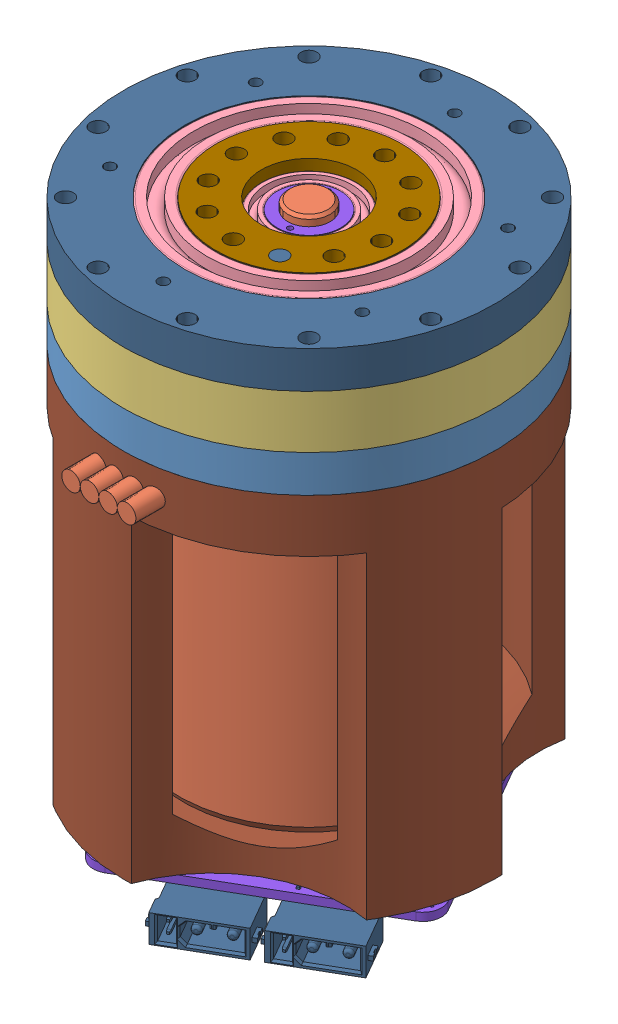
SolidWorks assembly Cycloidal_5065, configuration Default. Lengths in mm.
Overall size (95.62 102.59 95.62).
212 component instances, 82 part files, 54 mates.
Components (placement in the parent):
- Motor_base_5065-1: Motor_base_5065 [Default] at (25.1788 43.6468 54.8039) size (70 7 70)
- Flipsky 270kV motor.stp-1: Flipsky 270kV motor.stp [Default] at (25.1788 -19.3532 54.8039) x (0 1 0) z (-0.707107 0 0.707107) size (90.7 57.87 57.75)
- Ring_pin_housing_5065-1: Ring_pin_housing_5065 [Default] at (25.1788 50.6468 54.8039) size (70 10 70)
- radial ball bearing_68_iso-1: radial ball bearing_68_iso [ISO 15 RBB - 378 - 20,SI,NC,20_68] at (25.1788 48.8968 54.8039) x (0 1 0) z (-0.19787 0 0.980228) size (3.5 12 12)
- Ring_pin_5065-1: Ring_pin_5065 [Default] at (53.0279 61.6863 57.7576) x (-0.997886 0 0.064993) z (0.064993 0 0.997886) size (13.84 14 13.84)
  - m2_pin-1: m2_pin [Default] at (4.7265 1.0395 10.5113) size (4 14 4)
  - Ball_bearing_4x10x4-1: Ball_bearing_4x10x4 [Default] at (4.7265 9.0395 10.5113) size (10 4 10)
  - Ball_bearing_4x10x4-2: Ball_bearing_4x10x4 [Default] at (4.7265 3.0395 10.5113) x (-0.837169 0 -0.546944) z (-0.546944 0 0.837169) size (10 4 10)
- Ring_pin_5065-2: Ring_pin_5065 [Default] at (53.721 61.6863 30.5426) x (-1 0 0) z (0 0 1) size (13.84 14 13.84)
  - m2_pin-1: m2_pin [Default] at (4.7265 1.0395 10.5113) size (4 14 4)
  - Ball_bearing_4x10x4-1: Ball_bearing_4x10x4 [Default] at (4.7265 9.0395 10.5113) size (10 4 10)
  - Ball_bearing_4x10x4-2: Ball_bearing_4x10x4 [Default] at (4.7265 3.0395 10.5113) x (-0.837169 0 -0.546944) z (-0.546944 0 0.837169) size (10 4 10)
- Ring_pin_5065-3: Ring_pin_5065 [Default] at (15.4727 61.6863 76.0894) x (-0.146403 0 0.989225) z (0.989225 0 0.146403) size (13.84 14 13.84)
  - m2_pin-1: m2_pin [Default] at (4.7265 1.0395 10.5113) size (4 14 4)
  - Ball_bearing_4x10x4-1: Ball_bearing_4x10x4 [Default] at (4.7265 9.0395 10.5113) size (10 4 10)
  - Ball_bearing_4x10x4-2: Ball_bearing_4x10x4 [Default] at (4.7265 3.0395 10.5113) x (-0.837169 0 -0.546944) z (-0.546944 0 0.837169) size (10 4 10)
- Ring_pin_5065-4: Ring_pin_5065 [Default] at (6.0896 61.6863 58.0426) x (-1 0 0) z (0 0 1) size (13.84 14 13.84)
  - m2_pin-1: m2_pin [Default] at (4.7265 1.0395 10.5113) size (4 14 4)
  - Ball_bearing_4x10x4-1: Ball_bearing_4x10x4 [Default] at (4.7265 9.0395 10.5113) size (10 4 10)
  - Ball_bearing_4x10x4-2: Ball_bearing_4x10x4 [Default] at (4.7265 3.0395 10.5113) x (-0.837169 0 -0.546944) z (-0.546944 0 0.837169) size (10 4 10)
- Ring_pin_5065-5: Ring_pin_5065 [Default] at (29.9053 61.6863 16.7926) x (-1 0 0) z (0 0 1) size (13.84 14 13.84)
  - m2_pin-1: m2_pin [Default] at (4.7265 1.0395 10.5113) size (4 14 4)
  - Ball_bearing_4x10x4-1: Ball_bearing_4x10x4 [Default] at (4.7265 9.0395 10.5113) size (10 4 10)
  - Ball_bearing_4x10x4-2: Ball_bearing_4x10x4 [Default] at (4.7265 3.0395 10.5113) x (-0.837169 0 -0.546944) z (-0.546944 0 0.837169) size (10 4 10)
- Ring_pin_5065-6: Ring_pin_5065 [Default] at (6.0896 61.6863 30.5426) x (-1 0 0) z (0 0 1) size (13.84 14 13.84)
  - m2_pin-1: m2_pin [Default] at (4.7265 1.0395 10.5113) size (4 14 4)
  - Ball_bearing_4x10x4-1: Ball_bearing_4x10x4 [Default] at (4.7265 9.0395 10.5113) size (10 4 10)
  - Ball_bearing_4x10x4-2: Ball_bearing_4x10x4 [Default] at (4.7265 3.0395 10.5113) x (-0.837169 0 -0.546944) z (-0.546944 0 0.837169) size (10 4 10)
- Eccentric_shaft_5065-1: Eccentric_shaft_5065 [Default] at (16.4306 47.0254 47.869) x (0.967578 0 -0.252572) z (0.252572 0 0.967578) size (14 15 12)
  - Eccentric_shaft_bot_5065-1: Eccentric_shaft_bot_5065 [Default] at (6.713 3.6214 8.9195) size (12 5 12)
  - Eccentric_shaft_top_5065-1: Eccentric_shaft_top_5065 [Default] at (6.713 13.6214 8.9195) size (12 5 12)
  - Eccentric_shaft_bot_5065-2: Eccentric_shaft_bot_5065 [Default] at (6.713 8.6214 8.9195) x (-1 0 0) z (0 0 -1) size (12 5 12)
- radial ball bearing_68_iso-2: radial ball bearing_68_iso [ISO 15 RBB - 1712 - 20,SI,NC,20_68] at (25.1788 63.6468 54.8039) x (0 1 0) z (0 0 1) size (4 18 18)
- radial ball bearing_68_iso-3: radial ball bearing_68_iso [ISO 15 RBB - 1712 - 20,SI,NC,20_68] at (26.1463 58.6468 54.5513) x (0 -1 0) z (0.979558 0 -0.201164) size (4 18 18)
- radial ball bearing_68_iso-4: radial ball bearing_68_iso [ISO 15 RBB - 1712 - 20,SI,NC,20_68] at (24.2112 53.6468 55.0564) x (0 1 0) z (0 0 1) size (4 18 18)
- OutPut_shaft_5065-1: OutPut_shaft_5065 [Default] at (25.1788 60.6468 54.8039) x (0.876098 0 -0.482134) z (0.482134 0 0.876098) size (35 7 35)
- Output_cover_5065-1: Output_cover_5065 [Default] at (25.1788 60.6468 54.8039) size (70 7 70)
- Motor_cover_5065-1: Motor_cover_5065 [Default] at (25.1788 43.6468 54.8039) x (-0.866025 0 0.5) z (0.5 0 0.866025) size (70 70 70)
- Cycloidal_discs_5065-3: Cycloidal_discs_5065 [Default] at (3.9569 27.0207 21.2343) x (0.99705 0 -0.076752) z (0.076752 0 0.99705) size (45.09 5 45.95)
  - Cycloidal_discs_5065-1: Cycloidal_discs_5065 [Default] at (17.5986 23.6261 35.277) size (45.09 5 45.95)
  - radial ball bearing_68_iso-1: radial ball bearing_68_iso [ISO 15 RBB - 274 - 14,SI,NC,14_68] at (10.5986 27.3761 23.1526) x (0 1 0) z (-0.544662 0 0.838655) size (2.5 7 7)
  - radial ball bearing_68_iso-2: radial ball bearing_68_iso [ISO 15 RBB - 274 - 14,SI,NC,14_68] at (24.5986 27.3761 23.1526) x (0 1 0) z (-0.544662 0 0.838655) size (2.5 7 7)
  - radial ball bearing_68_iso-3: radial ball bearing_68_iso [ISO 15 RBB - 274 - 14,SI,NC,14_68] at (31.5986 27.3761 35.277) x (0 1 0) z (-0.544662 0 0.838655) size (2.5 7 7)
  - radial ball bearing_68_iso-4: radial ball bearing_68_iso [ISO 15 RBB - 274 - 14,SI,NC,14_68] at (24.5986 27.3761 47.4013) x (0 1 0) z (-0.544662 0 0.838655) size (2.5 7 7)
  - radial ball bearing_68_iso-5: radial ball bearing_68_iso [ISO 15 RBB - 274 - 14,SI,NC,14_68] at (10.5986 27.3761 47.4013) x (0 1 0) z (-0.544662 0 0.838655) size (2.5 7 7)
  - radial ball bearing_68_iso-6: radial ball bearing_68_iso [ISO 15 RBB - 274 - 14,SI,NC,14_68] at (3.5986 27.3761 35.277) x (0 1 0) z (-0.544662 0 0.838655) size (2.5 7 7)
- Cycloidal_discs_5065-5: Cycloidal_discs_5065 [Default] at (64.9013 32.0207 61.778) x (-0.602874 0 0.797837) z (-0.797837 0 -0.602874) size (45.09 5 45.95)
  - Cycloidal_discs_5065-1: Cycloidal_discs_5065 [Default] at (17.5986 23.6261 35.277) size (45.09 5 45.95)
  - radial ball bearing_68_iso-1: radial ball bearing_68_iso [ISO 15 RBB - 274 - 14,SI,NC,14_68] at (10.5986 27.3761 23.1526) x (0 1 0) z (-0.544662 0 0.838655) size (2.5 7 7)
  - radial ball bearing_68_iso-2: radial ball bearing_68_iso [ISO 15 RBB - 274 - 14,SI,NC,14_68] at (24.5986 27.3761 23.1526) x (0 1 0) z (-0.544662 0 0.838655) size (2.5 7 7)
  - radial ball bearing_68_iso-3: radial ball bearing_68_iso [ISO 15 RBB - 274 - 14,SI,NC,14_68] at (31.5986 27.3761 35.277) x (0 1 0) z (-0.544662 0 0.838655) size (2.5 7 7)
  - radial ball bearing_68_iso-4: radial ball bearing_68_iso [ISO 15 RBB - 274 - 14,SI,NC,14_68] at (24.5986 27.3761 47.4013) x (0 1 0) z (-0.544662 0 0.838655) size (2.5 7 7)
  - radial ball bearing_68_iso-5: radial ball bearing_68_iso [ISO 15 RBB - 274 - 14,SI,NC,14_68] at (10.5986 27.3761 47.4013) x (0 1 0) z (-0.544662 0 0.838655) size (2.5 7 7)
  - radial ball bearing_68_iso-6: radial ball bearing_68_iso [ISO 15 RBB - 274 - 14,SI,NC,14_68] at (3.5986 27.3761 35.277) x (0 1 0) z (-0.544662 0 0.838655) size (2.5 7 7)
- radial ball bearing_68_iso-5: radial ball bearing_68_iso [ISO 15 RBB - 274 - 14,SI,NC,14_68] at (25.1788 51.8968 54.8039) x (0 1 0) z (0.001306 0 0.999999) size (2.5 7 7)
- foc-motor-controller.step-1: foc-motor-controller.step [Default] at (25.1788 -28.1532 54.8039) x (-0.5 0 -0.866025) z (0 -1 0) size (57.23 50 8.13)
  - RTA0040B.step-1: RTA0040B.step [Default] at (12.5014 -1.6986 1.595) x (-0.707107 -0.707107 0) z (0 0 1) size (6 6 1)
    - FRAME.step-1: FRAME.step [Default] x (1 0 0) z (0 -1 0) size (6 0.2 6)
      - SOLID.step-1: SOLID.step [Default] at origin size (0.4 0.2 0.22)
      - SOLID-0.step-1: SOLID-0.step [Default] at origin size (0.4 0.2 0.22)
      - SOLID-1.step-1: SOLID-1.step [Default] at origin size (0.4 0.2 0.22)
      - SOLID-2.step-1: SOLID-2.step [Default] at origin size (0.4 0.2 0.22)
      - SOLID-3.step-1: SOLID-3.step [Default] at origin size (0.4 0.2 0.22)
      - SOLID-4.step-1: SOLID-4.step [Default] at origin size (0.4 0.2 0.22)
      - SOLID-5.step-1: SOLID-5.step [Default] at origin size (0.4 0.2 0.22)
      - SOLID-6.step-1: SOLID-6.step [Default] at origin size (0.4 0.2 0.22)
      - SOLID-7.step-1: SOLID-7.step [Default] at origin size (0.4 0.2 0.22)
      - SOLID-8.step-1: SOLID-8.step [Default] at origin size (0.4 0.2 0.22)
      - SOLID-9.step-1: SOLID-9.step [Default] at origin size (0.22 0.2 0.4)
      - SOLID-10.step-1: SOLID-10.step [Default] at origin size (0.22 0.2 0.4)
      - SOLID-11.step-1: SOLID-11.step [Default] at origin size (0.22 0.2 0.4)
      - SOLID-12.step-1: SOLID-12.step [Default] at origin size (0.22 0.2 0.4)
      - SOLID-13.step-1: SOLID-13.step [Default] at origin size (0.22 0.2 0.4)
      - SOLID-14.step-1: SOLID-14.step [Default] at origin size (0.22 0.2 0.4)
      - SOLID-15.step-1: SOLID-15.step [Default] at origin size (0.22 0.2 0.4)
      - SOLID-16.step-1: SOLID-16.step [Default] at origin size (0.22 0.2 0.4)
      - SOLID-17.step-1: SOLID-17.step [Default] at origin size (4.15 0.2 4.15)
      - SOLID-18.step-1: SOLID-18.step [Default] at origin size (0.28 0.1 0.28)
      - SOLID-19.step-1: SOLID-19.step [Default] at origin size (0.28 0.1 0.28)
      - SOLID-20.step-1: SOLID-20.step [Default] at origin size (0.28 0.1 0.28)
      - SOLID-21.step-1: SOLID-21.step [Default] at origin size (0.28 0.1 0.28)
      - SOLID-22.step-1: SOLID-22.step [Default] at origin size (0.4 0.2 0.22)
      - SOLID-23.step-1: SOLID-23.step [Default] at origin size (0.4 0.2 0.22)
      - SOLID-24.step-1: SOLID-24.step [Default] at origin size (0.4 0.2 0.22)
      - SOLID-25.step-1: SOLID-25.step [Default] at origin size (0.4 0.2 0.22)
      - SOLID-26.step-1: SOLID-26.step [Default] at origin size (0.4 0.2 0.22)
      - SOLID-27.step-1: SOLID-27.step [Default] at origin size (0.4 0.2 0.22)
      - SOLID-28.step-1: SOLID-28.step [Default] at origin size (0.4 0.2 0.22)
      - SOLID-29.step-1: SOLID-29.step [Default] at origin size (0.4 0.2 0.22)
      - SOLID-30.step-1: SOLID-30.step [Default] at origin size (0.4 0.2 0.22)
      - SOLID-31.step-1: SOLID-31.step [Default] at origin size (0.4 0.2 0.22)
      - SOLID-32.step-1: SOLID-32.step [Default] at origin size (0.22 0.2 0.4)
      - SOLID-33.step-1: SOLID-33.step [Default] at origin size (0.22 0.2 0.4)
      - SOLID-34.step-1: SOLID-34.step [Default] at origin size (0.22 0.2 0.4)
      - SOLID-35.step-1: SOLID-35.step [Default] at origin size (0.22 0.2 0.4)
      - SOLID-36.step-1: SOLID-36.step [Default] at origin size (0.22 0.2 0.4)
      - SOLID-37.step-1: SOLID-37.step [Default] at origin size (0.22 0.2 0.4)
      - SOLID-38.step-1: SOLID-38.step [Default] at origin size (0.22 0.2 0.4)
      - SOLID-39.step-1: SOLID-39.step [Default] at origin size (0.22 0.2 0.4)
      - SOLID-40.step-1: SOLID-40.step [Default] at origin size (0.22 0.2 0.4)
      - SOLID-41.step-1: SOLID-41.step [Default] at origin size (0.22 0.2 0.4)
      - SOLID-42.step-1: SOLID-42.step [Default] at origin size (0.22 0.2 0.4)
      - SOLID-43.step-1: SOLID-43.step [Default] at origin size (0.22 0.2 0.4)
    - BODY.step-1: BODY.step [Default] at (0 0 0.025) x (1 0 0) z (0 -1 0) size (6 0.97 6)
  - Resonator_SMD_Murata_CSTxExxV-3Pin_3.0x1.1mm.step-1: Resonator_SMD_Murata_CSTxExxV-3Pin_3.0x1.1mm.step [Default] at (1.8 -7 1.595) x (0 1 0) z (0 0 1) size (3.2 1.35 0.9)
  - C_0603_1608Metric.step-1: C_0603_1608Metric.step [Default] at (6.2 -16.8 1.595) x (0 -1 0) z (0 0 1) size (1.6 0.8 0.8)
  - R_0603_1608Metric.step-1: R_0603_1608Metric.step [Default] at (11.8 -7.375 1.595) x (0 1 0) z (0 0 1) size (1.6 0.8 0.45)
  - R_0603_1608Metric.step-2: R_0603_1608Metric.step [Default] at (13.8 -16.8 1.595) x (0 1 0) z (0 0 1) size (1.6 0.8 0.45)
  - R_0603_1608Metric.step-3: R_0603_1608Metric.step [Default] at (18.1 -5.36 1.595) size (1.6 0.8 0.45)
  - C_0603_1608Metric.step-2: C_0603_1608Metric.step [Default] at (2.6 -0.5 1.595) x (0 -1 0) z (0 0 1) size (1.6 0.8 0.8)
  - R_0603_1608Metric.step-4: R_0603_1608Metric.step [Default] at (14.6 -11.3 1.595) x (0 1 0) z (0 0 1) size (1.6 0.8 0.45)
  - L_APV_ANR4020.step-1: L_APV_ANR4020.step [Default] at (22.3 -13.7 1.595) x (0 -1 0) z (0 0 1) size (4.02 4 2)
  - C_0603_1608Metric.step-3: C_0603_1608Metric.step [Default] at (0.3 -12.6 1.595) x (-1 0 0) z (0 0 1) size (1.6 0.8 0.8)
  - C_1206_3216Metric.step-1: C_1206_3216Metric.step [Default] at (15.7 11 1.595) x (0 1 0) z (0 0 1) size (3.2 1.6 1.6)
  - C_0603_1608Metric.step-4: C_0603_1608Metric.step [Default] at (0.3 -9.6 1.595) size (1.6 0.8 0.8)
  - R_0603_1608Metric.step-5: R_0603_1608Metric.step [Default] at (12.3 -16.8 1.595) x (0 1 0) z (0 0 1) size (1.6 0.8 0.45)
  - C_0603_1608Metric.step-5: C_0603_1608Metric.step [Default] at (-0.3 -16.6 1.595) x (0 1 0) z (0 0 1) size (1.6 0.8 0.8)
  - R_0603_1608Metric.step-6: R_0603_1608Metric.step [Default] at (10.9 4.1 1.595) size (1.6 0.8 0.45)
  - C_1206_3216Metric.step-2: C_1206_3216Metric.step [Default] at (6.3 11 1.595) x (0 1 0) z (0 0 1) size (3.2 1.6 1.6)
  - XT30PW_2_2_-M.G.B.step-1: XT30PW_2_2_-M.G.B.step [Default] at (-20.5 9.5 1.595) x (0 -1 0) z (-1 0 0) size (15.5 7.1 12.53)
  - R_0603_1608Metric.step-7: R_0603_1608Metric.step [Default] at (0.3 -11.1 1.595) size (1.6 0.8 0.45)
  - C_0603_1608Metric.step-6: C_0603_1608Metric.step [Default] at (19 -0.4 1.595) x (-0.707107 -0.707107 0) z (0 0 1) size (1.6 0.8 0.8)
  - C_1206_3216Metric.step-3: C_1206_3216Metric.step [Default] at (13.3 11 1.595) x (0 1 0) z (0 0 1) size (3.2 1.6 1.6)
  - R_0603_1608Metric.step-8: R_0603_1608Metric.step [Default] at (10.2 -7.375 1.595) x (0 -1 0) z (0 0 1) size (1.6 0.8 0.45)
  - JST_GH_SM08B-GHS-TB_1x08-1MP_P1.25mm_Horizontal.step-1: JST_GH_SM08B-GHS-TB_1x08-1MP_P1.25mm_Horizontal.step [Default] at (10 -22 1.595) size (13.25 4.95 4.25)
  - C_1206_3216Metric.step-4: C_1206_3216Metric.step [Default] at (-12.3 11 1.595) x (0 1 0) z (0 0 1) size (3.2 1.6 1.6)
  - JST_GH_SM06B-GHS-TB_1x06-1MP_P1.25mm_Horizontal.step-1: JST_GH_SM06B-GHS-TB_1x06-1MP_P1.25mm_Horizontal.step [Default] at (-4.3 -22 1.595) size (10.75 4.95 4.25)
  - C_0603_1608Metric.step-7: C_0603_1608Metric.step [Default] at (7.3 -4.5 1.595) x (-1 0 0) z (0 0 1) size (1.6 0.8 0.8)
  - R_0603_1608Metric.step-9: R_0603_1608Metric.step [Default] at (18.1 -3.86 1.595) x (-1 0 0) z (0 0 1) size (1.6 0.8 0.45)
  - C_1206_3216Metric.step-5: C_1206_3216Metric.step [Default] at (22.6794 -1.2206 1.595) x (0.707107 -0.707107 0) z (0 0 1) size (3.2 1.6 1.6)
  - R_Array_Convex_4x0402.step-1: R_Array_Convex_4x0402.step [Default] at (6.8 -2.5 1.595) size (1 2 0.35)
  - R_0603_1608Metric.step-10: R_0603_1608Metric.step [Default] at (7.7 -16.8 1.595) x (0 -1 0) z (0 0 1) size (1.6 0.8 0.45)
  - C_1206_3216Metric.step-6: C_1206_3216Metric.step [Default] at (8.7 11 1.595) x (0 1 0) z (0 0 1) size (3.2 1.6 1.6)
  - C_0603_1608Metric.step-8: C_0603_1608Metric.step [Default] at (16.1 -11.3 1.595) x (0 1 0) z (0 0 1) size (1.6 0.8 0.8)
  - SOT-23-5.step-1: SOT-23-5.step [Default] at (-3.1 -16.6 1.595) x (-1 0 0) z (0 0 1) size (2.8 2.9 1.55)
  - C_0603_1608Metric.step-9: C_0603_1608Metric.step [Default] at (17.8 -13.6 1.595) size (1.6 0.8 0.8)
  - R_0603_1608Metric.step-11: R_0603_1608Metric.step [Default] at (-11.5 -20.3875 1.595) x (0 -1 0) z (0 0 1) size (1.6 0.8 0.45)
  - C_0603_1608Metric.step-10: C_0603_1608Metric.step [Default] at (-12.4 2.3 1.595) x (0 1 0) z (0 0 1) size (1.6 0.8 0.8)
  - C_1206_3216Metric.step-7: C_1206_3216Metric.step [Default] at (18 11 1.595) x (0 1 0) z (0 0 1) size (3.2 1.6 1.6)
  - R_0603_1608Metric.step-12: R_0603_1608Metric.step [Default] at (-10.8105 -14.9971 1.595) x (-1 0 0) z (0 0 1) size (1.6 0.8 0.45)
  - C_0603_1608Metric.step-11: C_0603_1608Metric.step [Default] at (-13.8 -9.4 1.595) x (-1 0 0) z (0 0 1) size (1.6 0.8 0.8)
  - R_0603_1608Metric.step-13: R_0603_1608Metric.step [Default] at (-23.15 -14.5 1.595) x (-1 0 0) z (0 0 1) size (1.6 0.8 0.45)
  - C_0603_1608Metric.step-12: C_0603_1608Metric.step [Default] at (1.1 -0.2 1.595) x (0 1 0) z (0 0 1) size (1.6 0.8 0.8)
  - D_0805_2012Metric.step-1: D_0805_2012Metric.step [Default] at (22.9 -9.6 1.595) x (0 1 0) z (0 0 1) size (2 1.27 0.8)
  - C_0603_1608Metric.step-13: C_0603_1608Metric.step [Default] at (-7.8 3.775 1.595) x (0 -1 0) z (0 0 1) size (1.6 0.8 0.8)
  - R_0603_1608Metric.step-14: R_0603_1608Metric.step [Default] at (-6.4 -12.825 1.595) x (0 1 0) z (0 0 1) size (1.6 0.8 0.45)
  - L_0603_1608Metric.step-1: L_0603_1608Metric.step [Default] at (-10.1 3 1.595) size (1.6 0.8 0.8)
  - C_0603_1608Metric.step-14: C_0603_1608Metric.step [Default] at (17.9 0.7 1.595) x (-0.707107 -0.707107 0) z (0 0 1) size (1.6 0.8 0.8)
  - HVSSOP-10.step-1: HVSSOP-10.step [Default] at (18.6 -9.6 1.595) x (0 -1 0) z (-1 0 0) size (4.9 1.1 3)
  - C_0603_1608Metric.step-15: C_0603_1608Metric.step [Default] at (7.9 4.1 1.595) x (-1 0 0) z (0 0 1) size (1.6 0.8 0.8)
  - C_0603_1608Metric.step-16: C_0603_1608Metric.step [Default] at (21.1 -9.6 1.595) x (0 -1 0) z (0 0 1) size (1.6 0.8 0.8)
  - R_0603_1608Metric.step-15: R_0603_1608Metric.step [Default] at (-10.8105 -11.9971 1.595) x (-1 0 0) z (0 0 1) size (1.6 0.8 0.45)
  - R_0603_1608Metric.step-16: R_0603_1608Metric.step [Default] at (-18.2 -17.4 1.595) size (1.6 0.8 0.45)
  - C_1206_3216Metric.step-8: C_1206_3216Metric.step [Default] at (-3 11 1.595) x (0 1 0) z (0 0 1) size (3.2 1.6 1.6)
  - R_0603_1608Metric.step-17: R_0603_1608Metric.step [Default] at (-16.9 -20.4 1.595) x (0 -1 0) z (0 0 1) size (1.6 0.8 0.45)
  - R_0603_1608Metric.step-18: R_0603_1608Metric.step [Default] at (-13.3 -20.3875 1.595) x (0 -1 0) z (0 0 1) size (1.6 0.8 0.45)
  - R_0603_1608Metric.step-19: R_0603_1608Metric.step [Default] at (-15.1 -20.3875 1.595) x (0 -1 0) z (0 0 1) size (1.6 0.8 0.45)
  - C_0603_1608Metric.step-17: C_0603_1608Metric.step [Default] at (15.5 -14.4 1.595) x (0 -1 0) z (0 0 1) size (1.6 0.8 0.8)
  - LED_0603_1608Metric.step-1: LED_0603_1608Metric.step [Default] at (-11.5 -23.3875 1.595) x (0 1 0) z (0 0 1) size (1.6 0.8 1.1)
  - C_0805_2012Metric.step-1: C_0805_2012Metric.step [Default] at (19.95 -17 1.595) size (2 1.25 1.25)
  - D_SMB.step-1: D_SMB.step [Default] at (-16.5 11.208 1.595) x (0 -1 0) z (0 0 1) size (5.3 3.55 2.15)
  - C_1206_3216Metric.step-9: C_1206_3216Metric.step [Default] at (-5.3 11 1.595) x (0 1 0) z (0 0 1) size (3.2 1.6 1.6)
  - XT30PW_2_2_-M.G.B.step-2: XT30PW_2_2_-M.G.B.step [Default] at (-20.5 -6.5 1.595) x (0 -1 0) z (-1 0 0) size (15.5 7.1 12.53)
  - C_1206_3216Metric.step-10: C_1206_3216Metric.step [Default] at (1.7 11 1.595) x (0 1 0) z (0 0 1) size (3.2 1.6 1.6)
  - C_1206_3216Metric.step-11: C_1206_3216Metric.step [Default] at (11 11 1.595) x (0 1 0) z (0 0 1) size (3.2 1.6 1.6)
  - C_0603_1608Metric.step-18: C_0603_1608Metric.step [Default] at (-6.3 3.775 1.595) x (0 -1 0) z (0 0 1) size (1.6 0.8 0.8)
  - C_0603_1608Metric.step-19: C_0603_1608Metric.step [Default] at (16.8686 1.7314 1.595) x (0.707107 0.707107 0) z (0 0 1) size (1.6 0.8 0.8)
  - C_0603_1608Metric.step-20: C_0603_1608Metric.step [Default] at (-15.0105 -11.1 1.595) size (1.6 0.8 0.8)
  - C_1206_3216Metric.step-12: C_1206_3216Metric.step [Default] at (-7.7 11 1.595) x (0 1 0) z (0 0 1) size (3.2 1.6 1.6)
  - C_0603_1608Metric.step-21: C_0603_1608Metric.step [Default] at (-18.2 -15.8 1.595) size (1.6 0.8 0.8)
  - C_0603_1608Metric.step-22: C_0603_1608Metric.step [Default] at (-2.1 -11.3 1.595) x (0 -1 0) z (0 0 1) size (1.6 0.8 0.8)
  - C_0603_1608Metric.step-23: C_0603_1608Metric.step [Default] at (-10.8105 -13.4971 1.595) size (1.6 0.8 0.8)
  - C_1206_3216Metric.step-13: C_1206_3216Metric.step [Default] at (4 11 1.595) x (0 1 0) z (0 0 1) size (3.2 1.6 1.6)
  - R_0603_1608Metric.step-20: R_0603_1608Metric.step [Default] at (16 -17.8 1.595) x (0 1 0) z (0 0 1) size (1.6 0.8 0.45)
  - Texas_S-PVSON-N8.step-1: Texas_S-PVSON-N8.step [Default] at (-14.4105 -13.7 1.595) x (-1 0 0) z (0 0 1) size (3 2.98 0.92)
  - C_1206_3216Metric.step-14: C_1206_3216Metric.step [Default] at (21 -2.9 1.595) x (0.707107 -0.707107 0) z (0 0 1) size (3.2 1.6 1.6)
  - C_0603_1608Metric.step-24: C_0603_1608Metric.step [Default] at (-5.9 -16.6 1.595) x (0 1 0) z (0 0 1) size (1.6 0.8 0.8)
  - C_0603_1608Metric.step-25: C_0603_1608Metric.step [Default] at (-3.1 -14.1 1.595) size (1.6 0.8 0.8)
  - R_0603_1608Metric.step-21: R_0603_1608Metric.step [Default] at (7.2 -7.375 1.595) x (0 -1 0) z (0 0 1) size (1.6 0.8 0.45)
  - C_1206_3216Metric.step-15: C_1206_3216Metric.step [Default] at (-0.7 11 1.595) x (0 1 0) z (0 0 1) size (3.2 1.6 1.6)
  - LQFP-64_10x10mm_P0.5mm.step-1: LQFP-64_10x10mm_P0.5mm.step [Default] at (-7 -4.5 1.595) x (-1 0 0) z (0 0 1) size (12 12 1.5)
  - C_0805_2012Metric.step-2: C_0805_2012Metric.step [Default] at (23.35 -17 1.595) x (-1 0 0) z (0 0 1) size (2 1.25 1.25)
  - C_0603_1608Metric.step-26: C_0603_1608Metric.step [Default] at (10.8 -16.8 1.595) x (0 -1 0) z (0 0 1) size (1.6 0.8 0.8)
  - R_0603_1608Metric.step-22: R_0603_1608Metric.step [Default] at (17.5 -17.8 1.595) x (0 -1 0) z (0 0 1) size (1.6 0.8 0.45)
  - C_1206_3216Metric.step-16: C_1206_3216Metric.step [Default] at (20.3 11 1.595) x (0 1 0) z (0 0 1) size (3.2 1.6 1.6)
  - R_0603_1608Metric.step-23: R_0603_1608Metric.step [Default] at (9.2 -16.8 1.595) x (0 -1 0) z (0 0 1) size (1.6 0.8 0.45)
  - C_1206_3216Metric.step-17: C_1206_3216Metric.step [Default] at (-10 11 1.595) x (0 1 0) z (0 0 1) size (3.2 1.6 1.6)
  - R_0603_1608Metric.step-24: R_0603_1608Metric.step [Default] at (17.8 -15.2 1.595) size (1.6 0.8 0.45)
  - C_1206_3216Metric.step-18: C_1206_3216Metric.step [Default] at (19.9 2.6 1.595) x (-0.707107 0.707107 0) z (0 0 1) size (3.2 1.6 1.6)
  - C_0603_1608Metric.step-27: C_0603_1608Metric.step [Default] at (13.4 -7.375 1.595) x (0 -1 0) z (0 0 1) size (1.6 0.8 0.8)
  - R_0603_1608Metric.step-25: R_0603_1608Metric.step [Default] at (8.7 -7.375 1.595) x (0 -1 0) z (0 0 1) size (1.6 0.8 0.45)
  - PQFN-8-EP_6x5mm_P1.27mm_Generic.step-1: PQFN-8-EP_6x5mm_P1.27mm_Generic.step [Default] at (4.9 14.4 -0.085) x (0 1 0) z (0 0 -1) size (6.15 5.15 1.09)
  - C_0805_2012Metric.step-3: C_0805_2012Metric.step [Default] at (-3 8.9 -0.085) x (0 1 0) z (0 0 -1) size (2 1.25 1.25)
  - C_0603_1608Metric.step-28: C_0603_1608Metric.step [Default] at (1.5 -4.3 -0.085) x (0 1 0) z (0 0 -1) size (1.6 0.8 0.8)
  - R_2512_6332Metric.step-1: R_2512_6332Metric.step [Default] at (2.1 8.6 -0.085) x (-1 0 0) z (0 0 -1) size (6.3 3.2 0.6)
  - C_0805_2012Metric.step-4: C_0805_2012Metric.step [Default] at (18.8 8.9 -0.085) x (0 1 0) z (0 0 -1) size (2 1.25 1.25)
  - C_0805_2012Metric.step-5: C_0805_2012Metric.step [Default] at (-5.2 8.901 -0.085) x (0 1 0) z (0 0 -1) size (2 1.25 1.25)
  - PQFN-8-EP_6x5mm_P1.27mm_Generic.step-2: PQFN-8-EP_6x5mm_P1.27mm_Generic.step [Default] at (16.9 14.6 -0.085) x (0 -1 0) z (0 0 -1) size (6.15 5.15 1.09)
  - PQFN-8-EP_6x5mm_P1.27mm_Generic.step-3: PQFN-8-EP_6x5mm_P1.27mm_Generic.step [Default] at (-1.1 14.6 -0.085) x (0 -1 0) z (0 0 -1) size (6.15 5.15 1.09)
  - R_0603_1608Metric.step-26: R_0603_1608Metric.step [Default] at (8.2 8.8 -0.085) x (0 1 0) z (0 0 -1) size (1.6 0.8 0.45)
  - R_2512_6332Metric.step-2: R_2512_6332Metric.step [Default] at (-10.3 8.601 -0.085) x (1 0 0) z (0 0 -1) size (6.3 3.2 0.6)
  - TSSOP-16_4.4x5mm_P0.65mm.step-1: TSSOP-16_4.4x5mm_P0.65mm.step [Default] at (0 0 -0.085) x (-1 0 0) z (0 0 -1) size (6.4 5 1.1)
  - C_0603_1608Metric.step-29: C_0603_1608Metric.step [Default] at (0 -4.25 -0.085) x (0 1 0) z (0 0 -1) size (1.6 0.8 0.8)
  - PQFN-8-EP_6x5mm_P1.27mm_Generic.step-4: PQFN-8-EP_6x5mm_P1.27mm_Generic.step [Default] at (10.9 14.4 -0.085) x (0 1 0) z (0 0 -1) size (6.15 5.15 1.09)
  - R_2512_6332Metric.step-3: R_2512_6332Metric.step [Default] at (13.7 8.6 -0.085) x (1 0 0) z (0 0 -1) size (6.3 3.2 0.6)
  - PQFN-8-EP_6x5mm_P1.27mm_Generic.step-5: PQFN-8-EP_6x5mm_P1.27mm_Generic.step [Default] at (-13.1 14.401 -0.085) x (0 1 0) z (0 0 -1) size (6.15 5.15 1.09)
  - C_0603_1608Metric.step-30: C_0603_1608Metric.step [Default] at (-1.5 -4.3 -0.085) x (0 -1 0) z (0 0 -1) size (1.6 0.8 0.8)
  - PQFN-8-EP_6x5mm_P1.27mm_Generic.step-6: PQFN-8-EP_6x5mm_P1.27mm_Generic.step [Default] at (-7.1 14.601 -0.085) x (0 -1 0) z (0 0 -1) size (6.15 5.15 1.09)
  - foc-motor-controller_PCB.step-1: foc-motor-controller_PCB.step [Default] at origin size (50 50 1.51)
- hex thin nut chamfered gradeab_iso-1: hex thin nut chamfered gradeab_iso [PreviewCfg] at (33.0483 -26.3532 25.4343) x (0.517651 0 -0.855592) z (0 1 0) size (5.5 6.35 1.8)
- m3_5065-1: m3_5065 [Default] at (31.9286 50.6468 67.0692) size (3 17 3)
- radial ball bearing_68_iso-7: radial ball bearing_68_iso [ISO 15 RBB - 1835 - 28,SI,NC,28_68] at (25.1788 64.1468 54.8039) x (0 1 0) z (0 0 1) size (7 47 47)
Mates (geometry in assembly coordinates):
- Coincident1: coincident anti-aligned: plane of Motor_base_5065-1 through (25.1788 43.6468 54.8039) normal (0 -1 0); plane of Flipsky 270kV motor.stp-1 through (25.1788 43.6468 54.8039) normal (0 1 0)
- Concentric1: concentric aligned: cylinder of Motor_base_5065-1 through (25.1788 50.6468 54.8039) axis (0 -1 0) radius 6; cylinder of Flipsky 270kV motor.stp-1 through (25.1788 43.6468 54.8039) axis (0 -1 0) radius 4
- Parallel1: parallel aligned: cylinder of Motor_base_5065-1 through (2.1978 50.6468 77.7848) axis (0 -1 0) radius 1.5; cylinder of Ring_pin_housing-1 through (2.1978 60.6468 77.7848) axis (0 -1 0) radius 1.5
- Concentric4: concentric aligned: cylinder of Motor_base_5065-1 through (1.3631 50.6468 68.5539) axis (0 -1 0) radius 1; cylinder of Ring_pin_housing-1 through (1.3631 60.6468 68.5539) axis (0 -1 0) radius 5.5
- Concentric5: concentric anti-aligned: cylinder of Motor_base_5065-1 through (25.1788 50.6468 54.8039) axis (0 -1 0) radius 6; cylinder of radial ball bearing_68_iso-1 through (25.1788 28.2593 54.8039) axis (0 1 0) radius 4
- Concentric6: concentric anti-aligned: cylinder of Motor_base_5065-1 through (48.9945 50.6468 68.5539) axis (0 -1 0) radius 1; cylinder of Ring_pin-1/m2_pin-1 through (48.9945 46.6468 68.5539) axis (0 1 0) radius 1
- Coincident3: coincident anti-aligned: plane of Motor_base_5065-1 through (25.1788 50.6468 54.8039) normal (0 1 0); plane of Ring_pin_5065-1/Ball_bearing_4x10x4-1 through (48.9945 50.6468 68.5539) normal (0 -1 0)
- Concentric7: concentric anti-aligned: cylinder of Motor_base_5065-1 through (48.9945 50.6468 41.0539) axis (0 -1 0) radius 1; cylinder of Ring_pin-2/m2_pin-1 through (48.9945 46.6468 41.0539) axis (0 1 0) radius 1
- Coincident4: coincident anti-aligned: plane of Motor_base_5065-1 through (25.1788 50.6468 54.8039) normal (0 1 0); plane of Ring_pin-2/Ball_bearing_4x10x4-1 through (48.9945 50.6468 41.0539) normal (0 -1 0)
- Coincident5: coincident anti-aligned: plane of Motor_base_5065-1 through (25.1788 50.6468 54.8039) normal (0 1 0); plane of Ring_pin_housing_5065-1 through (25.1788 50.6468 54.8039) normal (0 -1 0)
- Concentric9: concentric anti-aligned: cylinder of Motor_base_5065-1 through (25.1788 50.6468 82.3039) axis (0 -1 0) radius 1; cylinder of Ring_pin_5065-3/m2_pin-1 through (25.1788 46.6468 82.3039) axis (0 1 0) radius 1
- Concentric26: concentric anti-aligned: line of Motor_base_5065-1 through (25.1788 50.6468 27.3039) axis (0 -1 0); cylinder of Ring_pin-5/m2_pin-1 through (25.1788 50.6468 27.3039) axis (0 1 0) radius 1
- Concentric11: concentric anti-aligned: cylinder of Motor_base_5065-1 through (1.3631 50.6468 41.0539) axis (0 -1 0) radius 1; cylinder of Ring_pin-6/m2_pin-1 through (1.3631 46.6468 41.0539) axis (0 1 0) radius 1
- Concentric12: concentric anti-aligned: cylinder of Motor_base_5065-1 through (1.3631 50.6468 68.5539) axis (0 -1 0) radius 1; cylinder of Ring_pin-4/m2_pin-1 through (1.3631 46.6468 68.5539) axis (0 1 0) radius 1
- Coincident8: coincident anti-aligned: plane of Motor_base_5065-1 through (25.1788 50.6468 54.8039) normal (0 1 0); plane of Ring_pin-4/Ball_bearing_4x10x4-1 through (1.3631 50.6468 68.5539) normal (0 -1 0)
- Coincident9: coincident anti-aligned: plane of Motor_base_5065-1 through (25.1788 50.6468 54.8039) normal (0 1 0); plane of Ring_pin-6/Ball_bearing_4x10x4-1 through (1.3631 50.6468 41.0539) normal (0 -1 0)
- Coincident10: coincident anti-aligned: plane of Motor_base_5065-1 through (25.1788 50.6468 54.8039) normal (0 1 0); plane of Ring_pin-5/Ball_bearing_4x10x4-1 through (25.1788 50.6468 27.3039) normal (0 -1 0)
- Coincident11: coincident anti-aligned: plane of Motor_base_5065-1 through (25.1788 50.6468 54.8039) normal (0 1 0); plane of Eccentric_shaft_5065-1/Eccentric_shaft_bot_5065-1 through (24.2112 50.6468 55.0564) normal (0 -1 0)
- Concentric13: concentric anti-aligned: cylinder of radial ball bearing_68_iso-1 through (25.1788 28.2593 54.8039) axis (0 1 0) radius 4; cylinder of Eccentric_shaft_5065-1/Eccentric_shaft_bot_5065-2 through (25.1788 60.6468 54.8039) axis (0 -1 0) radius 4
- Concentric14: concentric anti-aligned: cylinder of Eccentric_shaft_5065-1/Eccentric_shaft_bot_5065-1 through (24.2112 55.6468 55.0564) axis (0 -1 0) radius 6; cylinder of radial ball bearing_68_iso-4 through (24.2112 33.0093 55.0564) axis (0 1 0) radius 6
- Coincident12: coincident aligned: plane of Eccentric_shaft_5065-1/Eccentric_shaft_bot_5065-1 through (24.2112 55.6468 55.0564) normal (0 1 0); circle of radial ball bearing_68_iso-4
- Concentric15: concentric anti-aligned: cylinder of ? through (26.1463 60.6468 54.5513) axis (0 -1 0) radius 6; line of radial ball bearing_68_iso-3 through (26.1463 54.0645 54.5513) axis (0 1 0)
- Coincident13: coincident aligned: circle of Eccentric_shaft-1/Eccentric_shaft_bot-2; plane of radial ball bearing_68_iso-3 through (24.7583 60.6468 47.7923) normal (0 1 0)
- Coincident14: coincident aligned: plane of Eccentric_shaft_5065-1/Eccentric_shaft_top_5065-1 through (25.1788 65.6468 54.8039) normal (0 1 0); circle of radial ball bearing_68_iso-2
- Concentric17: concentric anti-aligned: cylinder of Eccentric_shaft_5065-1/Eccentric_shaft_bot_5065-1 through (25.1788 55.6468 54.8039) axis (0 -1 0) radius 4; cylinder of radial ball bearing_68_iso-2 through (25.1788 43.0093 54.8039) axis (0 1 0) radius 6
- Concentric21: concentric anti-aligned: cylinder of radial ball bearing_68_iso-2 through (25.1788 43.0093 54.8039) axis (0 1 0) radius 9; cylinder of OutPut_shaft_5065-1 through (25.1788 67.6468 54.8039) axis (0 -1 0) radius 9
- Coincident20: coincident aligned: plane of Ring_pin_housing_5065-1 through (25.1788 60.6468 54.8039) normal (0 1 0); circle of Output_cover_5065-1
- Concentric24: concentric aligned: cylinder of Ring_pin_housing-1 through (2.1978 60.6468 77.7848) axis (0 -1 0) radius 1.5; cylinder of Output_cover_5065-1 through (2.1978 67.6468 77.7848) axis (0 -1 0) radius 1.5
- Coincident33: coincident aligned: plane of OutPut_shaft_5065-1 through (25.1788 67.6468 54.8039) normal (0 1 0); plane of Output_cover_5065-1 through (25.1788 67.6468 54.8039) normal (0 1 0)
- Concentric27: concentric aligned: cylinder of Flipsky 270kV motor.stp-1 through (25.1788 6.5468 54.8039) axis (0 1 0) radius 24.75; cylinder of Motor_cover_5065-1 through (25.1788 -21.3532 54.8039) axis (0 1 0) radius 30
- Coincident38: coincident aligned: plane of radial ball bearing_68_iso-4 through (15.4112 55.6468 55.0564) normal (0 1 0); plane of Cycloidal_discs_5065-3/Cycloidal_discs_5065-1 through (25.8664 55.6468 77.6141) normal (0 1 0)
- Concentric31: concentric anti-aligned: cylinder of radial ball bearing_68_iso-3 through (26.1463 79.2843 54.5513) axis (0 -1 0) radius 9; circle of Cycloidal_discs_5065-5/Cycloidal_discs_5065-1
- Coincident39: coincident aligned: plane of radial ball bearing_68_iso-3 through (24.5169 60.6468 46.6169) normal (0 1 0); plane of Cycloidal_discs_5065-5/Cycloidal_discs_5065-1 through (8.1495 60.6468 40.8508) normal (0 1 0)
- Concentric32: concentric anti-aligned: circle of radial ball bearing_68_iso-4; cylinder of Cycloidal_discs_5065-3/Cycloidal_discs_5065-1 through (24.2112 55.6468 55.0564) axis (0 -1 0) radius 9
- Concentric33: concentric anti-aligned: cylinder of OutPut_shaft_5065-1 through (25.1788 67.6468 54.8039) axis (0 -1 0) radius 17.5; cylinder of radial ball bearing_68_iso-5 through (25.1788 31.2593 54.8039) axis (0 1 0) radius 2
- Concentric34: concentric anti-aligned: cylinder of Motor_cover_5065-1 through (54.5483 -22.3532 62.6734) axis (0 -1 0) radius 1.5; cylinder of foc-motor-controller.step-1/foc-motor-controller_PCB.step-1 through (54.5483 -28.1072 62.6734) axis (0 1 0) radius 1.6
- Concentric35: concentric anti-aligned: cylinder of Motor_cover_5065-1 through (-4.1908 -22.3532 46.9343) axis (0 -1 0) radius 1.5; cylinder of foc-motor-controller.step-1/foc-motor-controller_PCB.step-1 through (-4.1908 -28.1072 46.9343) axis (0 1 0) radius 1.6
- Concentric36: concentric anti-aligned: cylinder of Motor_cover_5065-1 through (33.0483 -22.3532 25.4343) axis (0 -1 0) radius 1.5; cylinder of hex thin nut chamfered gradeab_iso-1 through (33.0483 -28.1532 25.4343) axis (0 1 0) radius 1.25
- Coincident43: coincident anti-aligned: plane of Motor_cover_5065-1 through (25.1788 -26.3532 54.8039) normal (0 -1 0); plane of hex thin nut chamfered gradeab_iso-1 through (30.3314 -26.3532 23.7906) normal (0 1 0)
- Coincident44: coincident anti-aligned: plane of foc-motor-controller.step-1/foc-motor-controller_PCB.step-1 through (25.1788 -28.1532 54.8039) normal (0 1 0); plane of hex thin nut chamfered gradeab_iso-1 through (30.3314 -28.1532 23.7906) normal (0 -1 0)
- Concentric37: concentric aligned: cylinder of OutPut_shaft_5065-1 through (31.9286 67.6468 67.0692) axis (0 -1 0) radius 1.5; cylinder of m3_5065-1 through (31.9286 67.6468 67.0692) axis (0 -1 0) radius 1.5
- Coincident45: coincident aligned: plane of Motor_base_5065-1 through (25.1788 50.6468 54.8039) normal (0 1 0); circle of m3_5065-1
- Tangent1: tangent aligned: cylinder of Cycloidal_discs_5065-5/radial ball bearing_68_iso-2 through (31.5995 38.7593 67.4456) axis (0 1 0) radius 2; cylinder of m3_5065-1 through (31.9286 67.6468 67.0692) axis (0 -1 0) radius 1.5
- Tangent5: tangent aligned: cylinder of Cycloidal_discs_5065-3/radial ball bearing_68_iso-4 through (32.1211 33.7593 66.6078) axis (0 1 0) radius 2; cylinder of m3_5065-1 through (31.9286 67.6468 67.0692) axis (0 -1 0) radius 1.5
- Concentric38: concentric anti-aligned: cylinder of OutPut_shaft_5065-1 through (25.1788 67.6468 54.8039) axis (0 -1 0) radius 17.5; cylinder of radial ball bearing_68_iso-7 through (25.1788 43.5093 54.8039) axis (0 1 0) radius 17.5
- Coincident46: coincident aligned: plane of Output_cover_5065-1 through (25.1788 67.6468 54.8039) normal (0 1 0); plane of radial ball bearing_68_iso-7 through (1.9788 67.6468 54.8039) normal (0 1 0)
- Coincident48: coincident aligned: plane of Ring_pin_housing_5065-1 through (25.1788 60.6468 54.8039) normal (0 1 0); plane of Ring_pin_5065-3/m2_pin-1 through (25.1788 60.6468 82.3039) normal (0 1 0)
- Coincident49: coincident anti-aligned: plane of Eccentric_shaft_5065-1/Eccentric_shaft_bot_5065-1 through (24.2112 50.6468 55.0564) normal (0 -1 0); circle of radial ball bearing_68_iso-5
- Coincident50: coincident aligned: plane of Motor_base_5065-1 through (25.1788 50.6468 54.8039) normal (0 1 0); plane of radial ball bearing_68_iso-1 through (19.3954 50.6468 53.6364) normal (0 1 0)
- Coincident51: coincident anti-aligned: plane of Motor_base_5065-1 through (25.1788 50.6468 54.8039) normal (0 1 0); plane of Eccentric_shaft_5065-1/Eccentric_shaft_bot_5065-1 through (24.2112 50.6468 55.0564) normal (0 -1 0)
- Concentric39: concentric aligned: cylinder of Motor_base_5065-1 through (25.1788 50.6468 54.8039) axis (0 -1 0) radius 35; cylinder of Ring_pin_housing_5065-1 through (25.1788 60.6468 54.8039) axis (0 -1 0) radius 35
- Coincident52: coincident anti-aligned: plane of Motor_base_5065-1 through (25.1788 43.6468 54.8039) normal (0 -1 0); plane of Motor_cover_5065-1 through (25.1788 43.6468 54.8039) normal (0 1 0)
- Concentric40: concentric anti-aligned: cylinder of Motor_base_5065-1 through (48.1597 50.6468 31.8229) axis (0 -1 0) radius 1.5; cylinder of Motor_cover_5065-1 through (48.1597 -21.3532 31.8229) axis (0 1 0) radius 1.5
- Concentric41: concentric aligned: cylinder of Ring_pin_housing_5065-1 through (25.1788 60.6468 54.8039) axis (0 -1 0) radius 35; cylinder of Output_cover_5065-1 through (25.1788 67.6468 54.8039) axis (0 -1 0) radius 35
